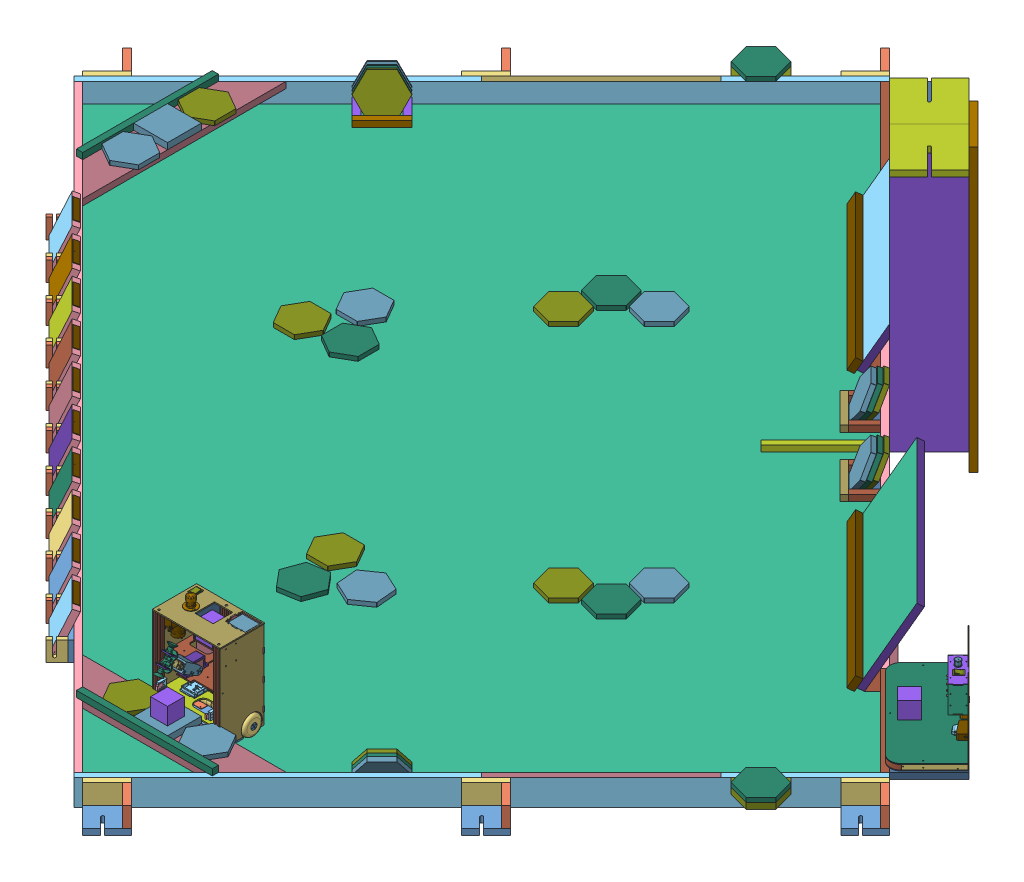
SolidWorks assembly conception_final_robot_autonome, configuration Default. Lengths in mm. (continued)
Components (placement in the parent): (continued)
- réplique-1: réplique [Default] at (173.8286 323.1947 656.2469) size (60 60 60)
- IBT-2 (module only)-1: IBT-2 (module only) [Default] at (112.5786 356.2835 564.3969) x (-1 0 0) z (0 0 1) size (51 40.62 49.7)
- IBT-2 (module only)-2: IBT-2 (module only) [Default] at (235.0786 361.6831 564.3969) size (51 40.62 49.7)
- support etage-1: support etage [Default] at (173.8286 272.8594 487.2468) x (1 0 0) z (0 1 0) size (19 14 15)
- support etage-2: support etage [Default] at (279.8286 272.9465 600.2469) x (-1 0 0) z (0 1 0) size (19 14 15)
- support etage-3: support etage [Default] at (67.8286 272.8594 600.2469) x (-1 0 0) z (0 1 0) size (19 14 15)
- réplique-3: réplique [Default] at (173.8286 480.6294 497.2468) size (60 60 60)
- support replique-1: support replique [Default] at (173.8286 446.6294 512.7469) x (-1 0 0) z (0 1 0) size (75 91 4)
- support etage-4: support etage [Default] at (173.8286 446.6294 487.2468) x (1 0 0) z (0 1 0) size (19 14 15)
- support etage-5: support etage [Default] at (163.8286 446.6294 477.2468) x (0 0 1) z (0 1 0) size (19 14 15)
- support etage-6: support etage [Default] at (183.8286 446.6294 477.2468) x (0 0 -1) z (0 1 0) size (19 14 15)
- support etage-7: support etage [Default] at (67.8286 379.2835 600.2469) x (-1 0 0) z (0 1 0) size (19 14 15)
- support etage-8: support etage [Default] at (279.8286 379.2835 600.2469) x (-1 0 0) z (0 1 0) size (19 14 15)
- support etage-9: support etage [Default] at (173.8286 379.2835 487.2468) x (1 0 0) z (0 1 0) size (19 14 15)
- etage lateral-1: etage lateral [Default] at (54.0286 394.8594 545.2469) x (0 0 -1) z (1 0 0) size (157 310 4)
- etage lateral-2: etage lateral [Default] at (289.6286 394.8594 545.2469) x (0 0 -1) z (1 0 0) size (157 310 4) (hidden)
- couvert arriere-1: couvert arriere [Default] at (184.7377 364.8594 463.2469) size (240 310 7)
- lipo battery-1: lipo battery [Default] at (255.0286 524.8594 497.2469) x (0 0 -1) z (0 -1 0) size (52 61 162)
- ventouse_final-1: ventouse_final [Default] at (157.7867 416.7859 702.1737) x (-0.271421 -0.541354 -0.79578) z (0.962461 -0.152666 -0.224416) size (30 42.25 32)
- ventouse_final-2: ventouse_final [Default] at (157.7867 490.4501 652.0613) x (-0.079274 0.560699 0.824216) z (0.996853 0.044589 0.065545) size (30 42.25 32)
- LM2596 DC to DC Buck Converter 3 A.STEP-1: LM2596 DC to DC Buck Converter 3 A.STEP [Default] at (274.0036 276.8594 498.8469) x (0 0 -1) z (1 0 0) size (43.2 15.15 21.25)
  - lm2596board.STEP-1: lm2596board.STEP [Default] at origin size (43.2 1.71 21.25)
  - smd100uF.STEP-1: smd100uF.STEP [Default] at (-17.25 2.55 0) x (0 0 -1) z (1 0 0) size (11.2 9.76 8.2)
  - smd220uF.STEP-1: smd220uF.STEP [Default] at (17.25 2.55 0) x (0 0 -1) z (1 0 0) size (11.2 9.76 8.2)
  - TrimmerW203.STEP-1: TrimmerW203.STEP [Default] at (4.6271 6.95 -9.1276) size (9.5 15.15 4.81)
  - smdS537diode.STEP-1: smdS537diode.STEP [Default] at (-9.35 1.75 8.875) x (-1 0 0) z (0 0 -1) size (6.5 2.06 2.5)
  - smdceramiccapacitor.STEP-1: smdceramiccapacitor.STEP [Default] at (-15 1.7 5.7969) x (0 0 1) z (-1 0 0) size (2.52 0.61 1.3)
  - smdceramiccapacitor.STEP-2: smdceramiccapacitor.STEP [Default] at (-1.3196 1.7 -5.2916) x (0 0 1) z (-1 0 0) size (2.52 0.61 1.3)
  - smdResistor331.STEP-1: smdResistor331.STEP [Default] at (-1.2696 1.7 -8.4665) x (0 0 1) z (-1 0 0) size (2.53 0.63 1.31)
  - smdResistor102.STEP-1: smdResistor102.STEP [Default] at (10.7771 1.7 -8.4665) x (0 0 -1) z (1 0 0) size (2.53 0.63 1.31)
  - smdLED.STEP-1: smdLED.STEP [Default] at (13.0521 1.75 -8.4701) x (0 0 -1) z (1 0 0) size (3.23 0.86 1.26)
  - smbInductor470.STEP-1: smbInductor470.STEP [Default] at (3.1271 2.1 3.175) size (12.5 7.41 12.5)
  - LM2596S.STEP-1: LM2596S.STEP [Default] at (-8.0627 1.8 -4.5407) size (9.8 4.61 14.95)
- e-stop 61-3440.stp-1: e-stop 61-3440.stp [Default] at (114.0286 514.8094 543.2469) x (-0.937891 0 -0.346929) z (0 1 0) size (43 43 76.4)
- couvert lateral replique-1: couvert lateral replique [Default] at (210.3286 485.7444 512.7469) x (0 0 1) z (-1 0 0) size (91 78.23 4)
- couvert lateral replique-2: couvert lateral replique [Default] at (141.3286 485.7444 512.7469) x (0 0 1) z (-1 0 0) size (91 78.23 4)
- profilé-1: profilé [Default] at (67.8286 364.8594 610.2469) x (1 0 0) z (0 -1 0) size (20 20 310)
- profilé-2: profilé [Default] at (279.8286 364.8594 610.2469) x (1 0 0) z (0 -1 0) size (20 20 310)
- profilé-3: profilé [Default] at (173.8286 364.8594 477.2469) x (1 0 0) z (0 -1 0) size (20 20 310)
- PompeVide-AirpoD2028B-12vdc-4: PompeVide-AirpoD2028B-12vdc [Défaut] at (77.3286 514.8594 552.1469) x (1 0 0) z (0 -1 0) size (38.6 62.4 92)
- roof-1: roof [Default] at (174.0286 528.8594 541.7469) x (1 0 0) z (0 -1 0) size (240 157 4)
- couvert lateral batterie-1: couvert lateral batterie [Default] at (216.0286 439.8594 497.2469) x (0 0 -1) z (1 0 0) size (63.8 174 4)
- couvert lateral batterie_2-1: couvert lateral batterie_2 [Default] at (255.0286 439.8594 531.2469) x (-1 0 0) z (0 0 -1) size (73.8 174 4)
- floor battery-1: floor battery [Default] at (252.5286 350.8594 497.0469) x (1 0 0) z (0 1 0) size (75.4 70.2 4)
- interrupteur principal-1: interrupteur principal [Défaut] at (76.5286 528.8594 489.2469) x (0 0 1) z (-1 0 0) size (32 33.35 25)
- support_ventouse-1: support_ventouse [Default] at (157.7867 440.3889 686.117) x (1 0 0) z (0 -0.826818 0.562469) size (35 26 4)
- support_ventouse-2: support_ventouse [Default] at (157.7867 470.1544 665.8681) x (1 0 0) z (0 -0.826818 0.562469) size (35 26 4)
- Assemblage1-1: Assemblage1 [Défaut] at (1585.9209 359.1947 -743.419) x (0.707107 0 0.707107) z (-0.707107 0 0.707107) size (440 246.17 210.2)
  - Pièce1-1: Pièce1 [Défaut] at origin size (440 156 3)
  - Pièce2-1: Pièce2 [Défaut] at (0 -85 105) x (-1 0 0) z (0 -1 0) size (439 210 3)
  - Part10 - Copie-1: Part10 - Copie [Default] at (-51.8676 -60.5031 49.9498) size (122.5 87.5 7.03)
  - Pièce9-1: Pièce9 [Défaut] at (-219.5 -76.5 104.5) x (0 0 -1) z (1 0 0) size (167 17 3)
  - Pièce6-2: Pièce6 [Défaut] at (-80 -76.5 207) size (359 17 3)
  - réplique-1: réplique [Default] at (0 -35 119.6611) size (60 60 60)
  - Pièce9-3: Pièce9 [Défaut] at (216.5 -76.5 104.5) x (0 0 -1) z (1 0 0) size (167 17 3)
  - Long Range SHARP IR Sensors - #GP2Y0A21YK0F-1: Long Range SHARP IR Sensors - #GP2Y0A21YK0F [Default] at (14.75 -35.3157 15.7) x (-1 0 0) z (0 0 1) size (44.5 18.9 13.5)
  - moraba3 3ordh-1: moraba3 3ordh [Défaut] at (-64.25 21.25 28) x (0 -1 0) z (1 0 0) size (93.5 53 3)
  - moraba3 3ordh-2: moraba3 3ordh [Défaut] at (61.25 21.25 27.8) x (0 -1 0) z (1 0 0) size (93.5 53 3)
  - moraba3 toul-2: moraba3 toul [Défaut] at (0 -25.5 28) x (1 0 0) z (0 1 0) size (128.5 53 3)
  - moraba3 toul loutaa-1: moraba3 toul loutaa [Défaut] at (0 65 28) x (1 0 0) z (0 1 0) size (128.5 53 3)
  - impr3d-1: impr3d [Défaut] at (0 -65 18) x (1 0 0) z (0 1 0) size (52 19 39.5)
  - FixAngle-1: FixAngle [Défaut] at (-216.5 -85 3) size (30 8 30)
  - FixAngle-2: FixAngle [Défaut] at (-61.25 -22.5 3) x (0 1 0) z (1 0 0) size (30 8 30)
  - FixAngle-3: FixAngle [Défaut] at (61.25 -22.5 3) x (-1 0 0) z (0 1 0) size (30 8 30)
  - FixAngle-4: FixAngle [Défaut] at (-61.25 65 3) x (1 0 0) z (0 -1 0) size (30 8 30)
  - FixAngle-5: FixAngle [Défaut] at (61.25 65 3) x (0 -1 0) z (-1 0 0) size (30 8 30)
  - FixAngle-9: FixAngle [Défaut] at (-61.25 -22.5 50.9) x (1 0 0) z (0 1 0) size (30 8 30)
  - FixAngle-10: FixAngle [Défaut] at (-61.25 65 50.9) x (0 -1 0) z (1 0 0) size (30 8 30)
  - FixAngle-11: FixAngle [Défaut] at (61.25 65 50.9) x (-1 0 0) z (0 -1 0) size (30 8 30)
  - FixAngle-12: FixAngle [Défaut] at (61.25 -22.5 50.9) x (0 1 0) z (-1 0 0) size (30 8 30)
  - arc_vitrine-1: arc_vitrine [Default] at (-219.5 -68 170) x (1 0 0) z (0 -1 0) size (50 50 17)
  - arc_vitrine-3: arc_vitrine [Default] at (179.5 -68 210) x (0 0 -1) z (0 -1 0) size (50 50 17)
  - support etage-1: support etage [Default] at (-216.5 -68 115) x (0 0 -1) z (0 1 0) size (19 14 15)
  - interrupteur principal-1: interrupteur principal [Défaut] at (13.25 68 26.5) x (0 0 -1) z (1 0 0) size (32 33.35 25)
  - FixAngle-13: FixAngle [Défaut] at (216.5 -85 3) x (0 0 1) z (-1 0 0) size (30 8 30)
  - support etage-3: support etage [Default] at (-77 -85 3) x (-1 0 0) z (0 -1 0) size (19 14 15)
  - support etage-4: support etage [Default] at (77 -85 3) x (-1 0 0) z (0 -1 0) size (19 14 15)
  - support etage-5: support etage [Default] at (216.5 -68 115) x (0 0 1) z (0 1 0) size (19 14 15)
  - Arduino UNO-1: Arduino UNO [Predeterminado] at (-140.4953 -85 41.7907) x (0 0 1) z (-1 0 0) size (74.8 15.1 53.3)
  - 5V One Channel Relay.step-1: 5V One Channel Relay.step [Default] at (-146.5 -85 84.8) x (0 0 1) z (-1 0 0) size (25.5 18.75 51)
  - support etage-6: support etage [Default] at (-22 -45.25 3) x (0 1 0) z (-1 0 0) size (19 14 15)
  - support etage-7: support etage [Default] at (22 -45.25 3) x (0 -1 0) z (1 0 0) size (19 14 15)
  - Force stop button-1: Force stop button [По умолчанию] at (-19.9998 66.9329 27.9999) x (0.906121 0 -0.423019) z (0 -1 0) size (20.79 20.79 48.92)
  - floor-1: floor [Default] at (0 -65 106.5) x (1 0 0) z (0 -1 0) size (439 207 3)
  - support etage-8: support etage [Default] at (0 -68 207) x (-1 0 0) z (0 1 0) size (19 14 15)
  - systeme de fixation-1: systeme de fixation [Défaut] at (0 -135 104.7444) x (-0.92707 0 -0.374889) z (-0.374889 0 0.92707) size (50.29 25 49.34)
  - fixation tige-1: fixation tige [Défaut] at (0 -85 104.7444) x (0.5 0 -0.866025) z (0.866025 0 0.5) size (13 55.5 15.01)
  - Long Range SHARP IR Sensors - #GP2Y0A21YK0F-2: Long Range SHARP IR Sensors - #GP2Y0A21YK0F [Default] at (122.0333 -35.3157 24.7506) x (-0.992278 0 -0.124035) z (-0.124035 0 0.992278) size (44.5 18.9 13.5)
  - support sharp lateral-1: support sharp lateral [Default] at (107.2359 -41.8157 3) size (60 20 29.34)
  - support sharp lateral-2: support sharp lateral [Default] at (-107.2359 -41.8157 3) x (-1 0 0) z (0 0 1) size (60 20 29.34)
  - Long Range SHARP IR Sensors - #GP2Y0A21YK0F-3: Long Range SHARP IR Sensors - #GP2Y0A21YK0F [Default] at (-92.7611 -35.3157 21.0916) x (-0.992278 0 0.124035) z (0.124035 0 0.992278) size (44.5 18.9 13.5)
- system wheel-1: system wheel [Default] at (267.4597 228.3737 520.7342) x (0 -0.852789 -0.522255) z (1 0 0) size (69.5 69.5 30.5)
  - part1-1: part1 [Default] at (0.5601 15.4113 33.6689) size (21.5 21.5 11)
  - part2-1: part2 [Default] at (0.5601 15.4113 5.1689) x (0 1 0) z (0 0 -1) size (21.5 21.5 18)
  - _gomme-1: _gomme [Default] at (0.5601 15.4113 11.6689) size (69.5 69.5 22)
- switch-1: switch [Default] at (84.2286 310.6027 623.2469) x (0 1 0) z (1 0 0) size (14 24 6)
- support_switch-1: support_switch [Default] at (77.8286 298.3527 609.7469) x (0 0 1) z (0 -1 0) size (29 9 24.5)
- switch-2: switch [Default] at (263.4286 310.6027 623.2469) x (0 -1 0) z (-1 0 0) size (14 24 6)
- support_switch-2: support_switch [Default] at (269.8286 322.8527 609.7469) x (0 0 1) z (0 1 0) size (29 9 24.5)
- system wheel-2: system wheel [Default] at (80.1976 227.4184 520.1492) x (0 0.852789 0.522255) z (-1 0 0) size (69.5 69.5 30.5)
  - part1-1: part1 [Default] at (0.5601 15.4113 33.6689) size (21.5 21.5 11)
  - part2-1: part2 [Default] at (0.5601 15.4113 5.1689) x (0 1 0) z (0 0 -1) size (21.5 21.5 18)
  - _gomme-1: _gomme [Default] at (0.5601 15.4113 11.6689) size (69.5 69.5 22)
- BillePorteuse-1: BillePorteuse [Défaut] at (173.8286 208.7594 609.7469) x (-0.837169 0 -0.546944) z (-0.546944 0 0.837169) size (31 21 31)
- etage lateral-3: etage lateral [Default] at (289.6286 394.8594 545.2469) x (0 0 -1) z (1 0 0) size (157 310 4)
- Baterijas testeris.step-1: Baterijas testeris.step [Default] at (200.7286 409.8594 471.7469) x (0 -1 0) z (1 0 0) size (41 12 24.1)
Mates (geometry in assembly coordinates):
- Coincident33: coincident anti-aligned: plane of étage 3-1 through (169.8286 383.2835 544.2469) normal (0 1 0); plane of Servo-1 through (150.2867 383.2835 566.2469) normal (0 -1 0)
- Concentric1: concentric anti-aligned: cylinder of Servo-1 through (146.7867 399.2835 597.2469) axis (1 0 0) radius 9.5; cylinder of bras_replique-1 through (146.7867 399.2835 597.2469) axis (-1 0 0) radius 12.5
- Coincident66: coincident anti-aligned: plane of Servo-1 through (146.7867 399.2835 597.2469) normal (-1 0 0); plane of bras_replique-1 through (146.7867 399.2835 597.2469) normal (1 0 0)
- Width3: width anti-aligned: plane of ##Servo_MG_996R-3 through (147.7867 431.8506 662.8986) normal (-1 0 0); plane of bras_replique-1 through (187.7867 431.8506 662.8986) normal (1 0 0); plane of ##Servo_MG_996R-3 through (146.7867 399.2835 597.2469) normal (1 0 0); plane of bras_replique-1 through (188.7867 399.2835 597.2469) normal (-1 0 0)
- Width4: width anti-aligned: plane of ##Servo_MG_996R-3 through (187.7867 431.8506 662.8986) normal (0 -0.826818 0.562469); plane of bras_replique-1 through (187.7867 448.3869 651.6492) normal (0 0.826818 -0.562469); plane of ##Servo_MG_996R-3 through (146.7867 412.5126 588.2474) normal (0 0.826818 -0.562469); plane of bras_replique-1 through (146.7867 386.0544 606.2464) normal (0 -0.826818 0.562469)
- Coincident67: coincident anti-aligned: plane of ##Servo_MG_996R-3 through (167.7867 435.844 650.9901) normal (0 -0.562469 -0.826818); plane of bras_replique-1 through (146.7867 435.844 650.9901) normal (0 0.562469 0.826818)
- Concentric5: concentric aligned: cylinder of ##Servo_MG_996R-3 through (157.7867 444.3373 663.475) axis (0 -0.562469 -0.826818) radius 3; cylinder of Access_HS-645_BrasRondPetitModele-1 through (157.7867 442.6499 660.9946) axis (0 -0.562469 -0.826818) radius 2.75
- Coincident71: coincident anti-aligned: plane of ##Servo_MG_996R-3 through (157.7867 444.3373 663.475) normal (0 0.562469 0.826818); plane of Access_HS-645_BrasRondPetitModele-1 through (160.5367 444.3373 663.475) normal (0 -0.562469 -0.826818)
- Width5: width anti-aligned: plane of support servo kbyr-1 through (151.5367 383.2835 566.2469) normal (0 0 1); plane of support servo kbyr-1 through (151.5367 405.2835 609.2469) normal (0 0 -1); plane of Servo-1 through (150.2867 383.2835 566.2469) normal (0 0 -1); plane of Servo-1 through (150.2867 383.2835 609.2469) normal (0 0 1)
- Width6: width aligned: plane of support servo kbyr-1 through (181.5367 409.2835 603.2469) normal (1 0 0); plane of support servo kbyr-1 through (151.5367 409.2835 603.2469) normal (-1 0 0); plane of Servo-1 through (182.7867 399.2835 587.7469) normal (1 0 0); plane of Servo-1 through (150.2867 399.2835 587.7469) normal (-1 0 0)
- Coincident75: coincident anti-aligned: plane of Servo-1 through (150.2867 415.2835 566.2469) normal (0 1 0); plane of support servo kbyr-1 through (151.5367 415.2835 566.2469) normal (0 -1 0)
- Distance1: distance = 15 mm: plane of support servo kbyr-1 through (151.5367 409.2835 614.2469) normal (0 0 1); plane of étage 3-1 through (289.8286 383.2835 629.2469) normal (0 0 1)
- Distance2: distance = 3 mm anti-aligned: plane of robot_sghyr-1/base_robot_sghyr-1 through (173.8286 209.8594 547.2469) normal (0 -1 0); plane of TABLE_2021.step-1/BaseTable.step-1/Ground.step-1 through (-179.7247 201.1947 -780.8956) normal (0 1 0)
- Distance3: distance = 3 mm anti-aligned: plane of étage 3-1 through (289.8286 383.2835 629.2469) normal (0 0 1); plane of TABLE_2021.step-1/Distributeurs.step-1/DistributeurCoin_1.step-1/Taquet.step-1 through (534.4531 249.1947 626.2469) normal (0 0 -1)
- Width7: width anti-aligned: plane of étage 3-1 through (289.8286 383.2835 467.2469) normal (1 0 0); plane of étage 3-1 through (57.8286 383.2835 467.2469) normal (-1 0 0); plane of TABLE_2021.step-1/Distributeurs.step-1/DistributeurCoin_1.step-1/SupportStatuette.step-1 through (113.8286 271.1947 626.2469) normal (-1 0 0); plane of TABLE_2021.step-1/Distributeurs.step-1/DistributeurCoin_1.step-1/SupportStatuette.step-1 through (233.8286 271.1947 746.2469) normal (1 0 0)
- Coincident81: coincident anti-aligned: plane of TABLE_2021.step-1/Distributeurs.step-1/DistributeurCoin_1.step-1/SupportStatuette.step-1 through (173.8286 293.1947 686.2469) normal (0 1 0); plane of réplique-1 through (143.8286 293.1947 716.2469) normal (0 -1 0)
- Width8: width anti-aligned: plane of réplique-1 through (203.8286 353.1947 716.2469) normal (1 0 0); plane of réplique-1 through (143.8286 353.1947 716.2469) normal (-1 0 0); plane of TABLE_2021.step-1/Distributeurs.step-1/DistributeurCoin_1.step-1/SupportStatuette.step-1 through (113.8286 271.1947 626.2469) normal (-1 0 0); plane of TABLE_2021.step-1/Distributeurs.step-1/DistributeurCoin_1.step-1/SupportStatuette.step-1 through (233.8286 271.1947 746.2469) normal (1 0 0)
- Width9: width aligned: plane of réplique-1 through (173.8286 323.1947 656.2469) normal (0 0 -1); plane of réplique-1 through (173.8286 323.1947 716.2469) normal (0 0 1); plane of TABLE_2021.step-1/Distributeurs.step-1/DistributeurCoin_1.step-1/Taquet.step-1 through (534.4531 249.1947 626.2469) normal (0 0 -1); plane of TABLE_2021.step-1/Distributeurs.step-1/DistributeurCoin_1.step-1/Taquet (1).step-1 through (414.4531 271.1947 746.2469) normal (0 0 -1)
- Parallel1: parallel aligned: plane of étage 3-1 through (169.8286 379.2835 544.2469) normal (0 -1 0); plane of IBT-2 (module only)-1 through (112.5786 354.6835 564.3969) normal (0 -1 0)
- Coincident87: coincident anti-aligned: plane of étage 3-1 through (169.8286 379.2835 544.2469) normal (0 -1 0); plane of IBT-2 (module only)-1 through (107.5231 379.2835 582.5719) normal (0 1 0)
- Parallel2: parallel aligned: plane of étage 3-1 through (57.8286 383.2835 467.2469) normal (-1 0 0); plane of IBT-2 (module only)-1 through (87.0786 356.2835 582.5719) normal (-1 0 0)
- Distance6: distance = 30 mm aligned: plane of étage 3-1 through (57.8286 383.2835 467.2469) normal (-1 0 0); plane of IBT-2 (module only)-1 through (87.8286 354.6835 586.7569) normal (-1 0 0)
- Width12: width aligned: plane of support etage-1 through (171.4786 257.8594 485.7468) normal (-1 0 0); plane of robot_sghyr-1/profilé-1 through (176.1786 257.8594 485.7468) normal (1 0 0); plane of support etage-1 through (168.3286 514.8594 483.8075) normal (0.707107 0 0.707107); plane of robot_sghyr-1/profilé-1 through (179.3286 514.8594 483.8075) normal (-0.707107 0 0.707107)
- Coincident90: coincident anti-aligned: plane of robot_sghyr-1/profilé-1 through (183.4286 514.8594 487.2468) normal (0 0 1); plane of support etage-1 through (183.3286 257.8594 487.2468) normal (0 0 -1)
- Coincident91: coincident anti-aligned: plane of robot_sghyr-1/etage electronique-1 through (173.8286 272.8594 547.2469) normal (0 -1 0); plane of support etage-1 through (183.3286 272.8594 487.2468) normal (0 1 0)
- Coincident94: coincident anti-aligned: plane of robot_sghyr-1/etage electronique-1 through (173.8286 272.8594 547.2469) normal (0 -1 0); plane of support etage-3 through (58.3286 272.8594 600.2469) normal (0 1 0)
- Width15: width aligned: plane of support replique-1 through (184.3286 450.6294 467.2469) normal (-1 0 0); plane of support replique-1 through (163.3286 450.6294 488.2469) normal (1 0 0); plane of robot_sghyr-1/profilé-1 through (163.8286 514.8594 486.8468) normal (-1 0 0); plane of robot_sghyr-1/profilé-1 through (183.8286 514.8594 486.8468) normal (1 0 0)
- Parallel3: parallel anti-aligned: plane of robot_sghyr-1/profilé-1 through (179.9286 514.8594 475.743) normal (0 1 0); plane of support replique-1 through (173.8286 466.6326 512.7469) normal (0 -1 0)
- Coincident95: coincident: plane of robot_sghyr-1/profilé-1 through (183.4286 514.8594 467.2468) normal (0 0 -1); plane of support replique-1 through (206.3286 470.6326 467.2469) normal (0 0 -1)
- Width18: width aligned: plane of support etage-6 through (182.3286 451.6326 479.5968) normal (0 0 1); plane of support etage-6 through (182.3286 451.6326 474.8968) normal (0 0 -1); plane of robot_sghyr-1/profilé-1 through (183.4286 514.8594 467.2468) normal (0 0 -1); plane of robot_sghyr-1/profilé-1 through (183.4286 514.8594 487.2468) normal (0 0 1)
- Coincident100: coincident anti-aligned: plane of robot_sghyr-1/profilé-1 through (183.8286 514.8594 486.8468) normal (1 0 0); plane of support etage-6 through (183.8286 451.6326 467.7468) normal (-1 0 0)
- Width19: width anti-aligned: plane of réplique-3 through (203.8286 510.6294 557.2468) normal (1 0 0); plane of réplique-3 through (143.8286 510.6294 557.2468) normal (-1 0 0); plane of support replique-1 through (141.3286 450.6294 558.2469) normal (-1 0 0); plane of support replique-1 through (206.3286 450.6294 558.2469) normal (1 0 0)
- Coincident102: coincident anti-aligned: plane of réplique-3 through (143.8286 450.6294 557.2468) normal (0 -1 0); plane of support replique-1 through (173.8286 450.6294 512.7469) normal (0 1 0)
- Coincident104: coincident anti-aligned: plane of étage 3-1 through (169.8286 379.2835 544.2469) normal (0 -1 0); plane of support etage-7 through (58.3286 379.2835 600.2469) normal (0 1 0)
- Coincident106: coincident anti-aligned: plane of étage 3-1 through (169.8286 379.2835 544.2469) normal (0 -1 0); plane of support etage-8 through (270.3286 379.2835 600.2469) normal (0 1 0)
- Width22: width anti-aligned: plane of support etage-9 through (176.1786 364.2835 485.7468) normal (1 0 0); plane of support etage-9 through (171.4786 364.2835 485.7468) normal (-1 0 0); plane of robot_sghyr-1/profilé-1 through (183.8286 514.8594 486.8468) normal (1 0 0); plane of robot_sghyr-1/profilé-1 through (163.8286 514.8594 486.8468) normal (-1 0 0)
- Coincident107: coincident anti-aligned: plane of robot_sghyr-1/profilé-1 through (164.2286 514.8594 487.2468) normal (0 0 1); plane of support etage-9 through (183.3286 364.2835 487.2468) normal (0 0 -1)
- Coincident108: coincident anti-aligned: plane of étage 3-1 through (169.8286 379.2835 544.2469) normal (0 -1 0); plane of support etage-9 through (183.3286 379.2835 487.2468) normal (0 1 0)
- Width23: width anti-aligned: plane of étage 3-1 through (57.8286 383.2835 467.2469) normal (-1 0 0); plane of étage 3-1 through (289.8286 383.2835 467.2469) normal (1 0 0); plane of robot_sghyr-1/base_robot_sghyr-1 through (258.8286 209.8594 537.2469) normal (1 0 0); plane of robot_sghyr-1/base_robot_sghyr-1 through (88.8286 209.8594 537.2469) normal (-1 0 0)
- Coincident112: coincident anti-aligned: plane of robot_sghyr-1/base_robot_sghyr-1 through (173.8286 214.8594 547.2469) normal (0 1 0); plane of etage lateral-1 through (58.0286 214.8594 620.2469) normal (0 -1 0)
- Coincident114: coincident aligned: plane of robot_sghyr-1/profilé-1 through (183.4286 514.8594 467.2468) normal (0 0 -1); plane of étage 3-1 through (289.8286 384.2835 467.2469) normal (0 0 -1)
- Coincident115: coincident anti-aligned: plane of robot_sghyr-1/base_robot_sghyr-1 through (173.8286 214.8594 547.2469) normal (0 1 0); plane of couvert arriere-1 through (53.8286 214.8594 467.2469) normal (0 -1 0)
- Coincident116: coincident aligned: plane of robot_sghyr-1/base_robot_sghyr-1 through (53.8286 214.8594 462.2469) normal (-1 0 0); plane of couvert arriere-1 through (53.8286 544.8594 467.2469) normal (-1 0 0)
- Coincident117: coincident anti-aligned: plane of couvert arriere-1 through (184.7377 364.8594 467.2469) normal (0 0 1); plane of robot_sghyr-1/profilé-1 through (183.4286 514.8594 467.2468) normal (0 0 -1)
- Coincident120: coincident anti-aligned: plane of robot_sghyr-1/etage electronique-1 through (173.8286 276.8594 547.2469) normal (0 1 0); plane of LM2596 DC to DC Buck Converter 3 A.STEP-1/lm2596board.STEP-1 through (274.0036 276.8594 498.8469) normal (0 -1 0)
- Distance7: distance = 5 mm anti-aligned: plane of LM2596 DC to DC Buck Converter 3 A.STEP-1/lm2596board.STEP-1 through (284.6286 278.5594 520.4469) normal (1 0 0); plane of etage lateral-2 through (289.6286 394.8594 545.2469) normal (-1 0 0)
- Distance8: distance = 10 mm anti-aligned: plane of couvert arriere-1 through (184.7377 364.8594 467.2469) normal (0 0 1); plane of LM2596 DC to DC Buck Converter 3 A.STEP-1/lm2596board.STEP-1 through (284.6286 278.5594 477.2469) normal (0 0 -1)
- Distance9: distance = 10 mm anti-aligned: plane of robot_sghyr-1/profilé-1 through (183.4286 514.8594 487.2468) normal (0 0 1); plane of réplique-3 through (173.8286 500.6326 497.2468) normal (0 0 -1)
- Coincident127: coincident anti-aligned: plane of couvert arriere-1 through (184.7377 364.8594 467.2469) normal (0 0 1); plane of couvert lateral replique-1 through (206.3286 524.8594 467.2469) normal (0 0 -1)
- Coincident130: coincident anti-aligned: plane of support replique-1 through (206.3286 450.6294 558.2469) normal (1 0 0); plane of couvert lateral replique-1 through (206.3286 485.7444 512.7469) normal (-1 0 0)
- Concentric9: concentric anti-aligned: cylinder of robot_sghyr-1/base_robot_sghyr-1 through (67.8286 214.8594 610.2469) axis (0 -1 0) radius 2.5; cylinder of profilé-1 through (67.8286 214.8594 610.2469) axis (0 1 0) radius 2.5
- Coincident131: coincident anti-aligned: plane of robot_sghyr-1/base_robot_sghyr-1 through (173.8286 214.8594 547.2469) normal (0 1 0); plane of profilé-1 through (66.3248 214.8594 616.3469) normal (0 -1 0)
- Concentric10: concentric anti-aligned: cylinder of robot_sghyr-1/base_robot_sghyr-1 through (173.8286 214.8594 477.2469) axis (0 -1 0) radius 2.5; cylinder of profilé-3 through (173.8286 214.8594 477.2469) axis (0 1 0) radius 2.5
- Coincident132: coincident anti-aligned: plane of robot_sghyr-1/base_robot_sghyr-1 through (173.8286 214.8594 547.2469) normal (0 1 0); plane of profilé-3 through (172.3248 214.8594 483.3469) normal (0 -1 0)
- Coincident133: coincident aligned: plane of etage lateral-2 through (293.6286 544.8594 620.2469) normal (0 0 1); plane of profilé-2 through (289.4286 214.8594 620.2469) normal (0 0 1)
- Coincident137: coincident anti-aligned: plane of etage lateral-2 through (289.6286 394.8594 545.2469) normal (-1 0 0); plane of couvert arriere-1 through (289.6286 255.0594 467.2469) normal (1 0 0)
- Coincident138: coincident aligned: plane of etage lateral-2 through (293.6286 544.8594 463.2469) normal (0 0 -1); plane of couvert arriere-1 through (184.7377 364.8594 463.2469) normal (0 0 -1)
- Coincident139: coincident anti-aligned: plane of robot_sghyr-1/etage electronique-1 through (289.8286 272.8594 467.2469) normal (0 0 -1); plane of couvert arriere-1 through (184.7377 364.8594 467.2469) normal (0 0 1)
- Coincident148: coincident anti-aligned: plane of PompeVide-AirpoD2028B-12vdc-1 through (289.6286 475.8594 595.2469) normal (1 0 0); plane of etage lateral-2 through (289.6286 394.8594 545.2469) normal (-1 0 0)
- Distance12: distance = 5 mm anti-aligned: plane of PompeVide-AirpoD2028B-12vdc-1 through (251.0286 475.8594 595.2469) normal (0 0 1); plane of profilé-2 through (270.2286 214.8594 600.2469) normal (0 0 -1)
- Coincident154: coincident anti-aligned: plane of profilé-1 through (66.3248 524.8594 616.3469) normal (0 1 0); plane of roof-1 through (174.0286 524.8594 541.7469) normal (0 -1 0)
- Coincident155: coincident aligned: plane of etage lateral-1 through (54.0286 394.8594 545.2469) normal (-1 0 0); plane of roof-1 through (54.0286 524.8594 620.2469) normal (-1 0 0)
- Coincident156: coincident aligned: plane of profilé-1 through (77.4286 214.8594 620.2469) normal (0 0 1); plane of roof-1 through (54.0286 524.8594 620.2469) normal (0 0 1)
- Width27: width anti-aligned: plane of roof-1 through (216.0286 524.8594 487.2469) normal (0 0 1); plane of roof-1 through (220.0286 524.8594 507.2469) normal (0 0 -1); plane of couvert lateral batterie-1 through (220.0286 528.8594 487.3469) normal (0 0 -1); plane of couvert lateral batterie-1 through (220.0286 524.8594 507.1469) normal (0 0 1)
- Coincident157: coincident anti-aligned: plane of roof-1 through (216.0286 524.8594 507.2469) normal (1 0 0); plane of couvert lateral batterie-1 through (216.0286 439.8594 497.2469) normal (-1 0 0)
- Coincident158: coincident aligned: plane of roof-1 through (174.0286 528.8594 541.7469) normal (0 1 0); plane of couvert lateral batterie-1 through (220.0286 528.8594 507.1469) normal (0 1 0)
- Width28: width anti-aligned: plane of couvert lateral batterie_2-1 through (264.9286 524.8594 527.2469) normal (1 0 0); plane of couvert lateral batterie_2-1 through (245.1286 528.8594 527.2469) normal (-1 0 0); plane of roof-1 through (245.0286 524.8594 531.2469) normal (1 0 0); plane of roof-1 through (265.0286 524.8594 527.2469) normal (-1 0 0)
- Coincident159: coincident aligned: plane of roof-1 through (174.0286 528.8594 541.7469) normal (0 1 0); plane of couvert lateral batterie_2-1 through (264.9286 528.8594 527.2469) normal (0 1 0)
- Coincident160: coincident anti-aligned: plane of roof-1 through (265.0286 524.8594 531.2469) normal (0 0 -1); plane of couvert lateral batterie_2-1 through (255.0286 439.8594 531.2469) normal (0 0 1)
- Width29: width aligned: plane of lipo battery-1 through (224.5286 362.8594 523.2469) normal (-1 0 0); plane of lipo battery-1 through (285.5286 362.8594 523.2469) normal (1 0 0); plane of roof-1 through (290.0286 524.8594 467.2469) normal (-1 0 0); plane of roof-1 through (220.0286 524.8594 507.2469) normal (1 0 0)
- Width30: width aligned: plane of roof-1 through (220.0286 524.8594 467.2469) normal (0 0 1); plane of roof-1 through (220.0286 524.8594 527.2469) normal (0 0 -1); plane of lipo battery-1 through (285.5286 362.8594 523.2469) normal (0 0 1); plane of lipo battery-1 through (285.5286 362.8594 471.2469) normal (0 0 -1)
- Concentric11: concentric aligned: cylinder of e-stop 61-3440.stp-1 through (114.0286 532.9094 543.2469) axis (0 1 0) radius 12; cylinder of roof-1 through (114.0286 524.8594 543.2469) axis (0 1 0) radius 7.5
- Coincident161: coincident anti-aligned: plane of e-stop 61-3440.stp-1 through (114.0286 528.8594 543.2469) normal (0 -1 0); plane of roof-1 through (174.0286 528.8594 541.7469) normal (0 1 0)
- Distance13: distance = 4 mm aligned: plane of lipo battery-1 through (255.0286 524.8594 497.2469) normal (0 1 0); plane of roof-1 through (174.0286 528.8594 541.7469) normal (0 1 0)
- Distance14: distance = 40 mm aligned: plane of IBT-2 (module only)-2 through (212.8286 363.2831 589.2469) normal (0 0 1); plane of étage 3-1 through (289.8286 383.2835 629.2469) normal (0 0 1)
- Coincident163: coincident anti-aligned: plane of couvert lateral batterie_2-1 through (289.9286 354.8594 527.2469) normal (0 -1 0); plane of floor battery-1 through (252.5286 354.8594 497.0469) normal (0 1 0)
- Coincident164: coincident aligned: plane of couvert lateral batterie-1 through (216.0286 439.8594 497.2469) normal (-1 0 0); plane of floor battery-1 through (216.0286 354.8594 467.2469) normal (-1 0 0)
- Coincident165: coincident anti-aligned: plane of couvert arriere-1 through (184.7377 364.8594 467.2469) normal (0 0 1); plane of floor battery-1 through (216.0286 354.8594 467.2469) normal (0 0 -1)
- Coincident166: coincident anti-aligned: plane of roof-1 through (174.0286 528.8594 541.7469) normal (0 1 0); plane of interrupteur principal-1 through (76.5286 528.8594 489.2469) normal (0 -1 0)
- Parallel4: parallel anti-aligned: plane of roof-1 through (54.0286 524.8594 620.2469) normal (-1 0 0); plane of interrupteur principal-1 through (89.0286 530.8594 473.2469) normal (1 0 0)
- Distance15: distance = 10 mm aligned: plane of interrupteur principal-1 through (64.0286 530.8594 473.2469) normal (0 0 -1); plane of roof-1 through (54.0286 524.8594 463.2469) normal (0 0 -1)
- Distance16: distance = 10 mm aligned: plane of interrupteur principal-1 through (64.0286 530.8594 473.2469) normal (-1 0 0); plane of roof-1 through (54.0286 524.8594 620.2469) normal (-1 0 0)
- Coincident173: coincident anti-aligned: plane of support_ventouse-1 through (162.7867 430.8945 679.2719) normal (0 -0.562469 -0.826818); plane of SUPPORT VENTOUSE-1 through (147.1896 426.7604 682.0842) normal (0 0.562469 0.826818)
- Concentric12: concentric anti-aligned: cylinder of ventouse_final-1 through (157.7867 416.7859 702.1737) axis (0 -0.826818 0.562469) radius 6.5; cylinder of support_ventouse-1 through (157.7867 437.0816 688.3669) axis (0 0.826818 -0.562469) radius 6.5
- Coincident174: coincident anti-aligned: plane of ventouse_final-1 through (157.7867 437.0816 688.3669) normal (0 0.826818 -0.562469); plane of support_ventouse-1 through (157.7867 437.0816 688.3669) normal (0 -0.826818 0.562469)
- Coincident175: coincident anti-aligned: plane of SUPPORT VENTOUSE-1 through (157.7867 442.9311 661.408) normal (-1 0 0); plane of support_ventouse-1 through (157.7867 440.3889 686.117) normal (1 0 0)
- Width31: width anti-aligned: plane of SUPPORT VENTOUSE-1 through (144.776 418.1266 678.282) normal (0 -0.826818 0.562469); plane of SUPPORT VENTOUSE-1 through (144.776 467.7357 644.5339) normal (0 0.826818 -0.562469); plane of bras_replique-1 through (146.7867 412.5126 588.2474) normal (0 0.826818 -0.562469); plane of bras_replique-1 through (146.7867 386.0544 606.2464) normal (0 -0.826818 0.562469)
- Concentric13: concentric aligned: cylinder of ventouse_final-2 through (157.7867 490.4501 652.0613) axis (0 0.826818 -0.562469) radius 6.5; cylinder of support_ventouse-2 through (157.7867 466.8471 668.118) axis (0 0.826818 -0.562469) radius 6.5
- Distance18: distance = 10 mm aligned: plane of support_ventouse-1 through (157.7867 437.0816 688.3669) normal (0 -0.826818 0.562469); plane of SUPPORT VENTOUSE-1 through (144.776 418.1266 678.282) normal (0 -0.826818 0.562469)
- Coincident181: coincident anti-aligned: plane of ventouse_final-2 through (157.7867 470.1544 665.8681) normal (0 -0.826818 0.562469); plane of support_ventouse-2 through (157.7867 470.1544 665.8681) normal (0 0.826818 -0.562469)
- Coincident182: coincident anti-aligned: plane of TABLE_2021.step-1/BaseTable.step-1/ExperimentZone.step-2 through (1515.2102 271.1947 -672.7083) normal (0 1 0); plane of Assemblage1-1/Pièce2-1 through (1511.6747 271.1947 -669.1728) normal (0 -1 0)
- Coincident184: coincident aligned: plane of TABLE_2021.step-1/BaseTable.step-1/ExperimentZone.step-2 through (1589.4564 271.1947 -739.8834) normal (0.707107 0 -0.707107); plane of Assemblage1-1/Pièce1-1 through (1585.9209 359.1947 -743.419) normal (0.707107 0 -0.707107)
- Width35: width anti-aligned: plane of TABLE_2021.step-1/BaseTable.step-1/ExperimentZone.step-2 through (1745.0199 271.1947 -584.32) normal (0.707107 0 0.707107); plane of Assemblage1-1/Pièce9-1 through (1285.4005 271.1947 -761.0966) normal (-0.707107 0 -0.707107); plane of TABLE_2021.step-1/BaseTable.step-1/ExperimentZone.step-2 through (1356.8183 282.6947 -824.7363) normal (-0.707107 0 -0.707107); plane of Assemblage1-1/Pièce9-2 through (1667.2382 350.1947 -513.6093) normal (0.707107 0 0.707107)
- Concentric14: concentric aligned: cylinder of ##Servo_MG_996R-3 through (157.7867 444.3373 663.475) axis (0 -0.562469 -0.826818) radius 3; cylinder of Access_HS-645_BrasRondPetitModele-1 through (157.7867 442.6499 660.9946) axis (0 -0.562469 -0.826818) radius 4.5
- Coincident187: coincident anti-aligned: plane of SUPPORT VENTOUSE-1 through (157.7867 442.9311 661.408) normal (-1 0 0); plane of Access_HS-645_BrasRondPetitModele-1 through (157.7867 442.6499 660.9946) normal (1 0 0)
- Coincident188: coincident anti-aligned: plane of SUPPORT VENTOUSE-1 through (135.3298 469.9855 647.8412) normal (0 -0.562469 -0.826818); plane of Access_HS-645_BrasRondPetitModele-1 through (161.5367 445.181 664.7152) normal (0 0.562469 0.826818)
- Concentric15: concentric aligned: cylinder of robot_sghyr-1/pololu-37D-encoder-1 through (273.8286 235.8594 507.2469) axis (-1 0 0) radius 3; cylinder of system wheel-1/accoupelement court-1 through (272.8286 235.8594 507.2469) axis (-1 0 0) radius 3
- Coincident189: coincident anti-aligned: plane of profilé-1 through (77.8286 214.8594 619.8469) normal (1 0 0); plane of support_switch-1 through (77.8286 322.8527 619.2469) normal (-1 0 0)
- Width39: width aligned: plane of switch-1 through (85.8286 317.6027 632.2469) normal (0 1 0); plane of switch-1 through (85.8286 303.6027 632.2469) normal (0 -1 0); plane of support_switch-1 through (77.8286 322.8527 619.2469) normal (0 1 0); plane of support_switch-1 through (77.8286 298.3527 619.2469) normal (0 -1 0)
- Parallel5: parallel aligned: plane of switch-1 through (85.8286 303.6027 614.2469) normal (0 0 -1); plane of support_switch-1 through (77.8286 298.3527 600.2469) normal (0 0 -1)
- Distance20: distance = 6 mm aligned: plane of robot_sghyr-1/base_robot_sghyr-1 through (293.8286 214.8594 632.2469) normal (0 0 1); plane of switch-1 through (89.8286 303.6027 638.2469) normal (0 0 1)
- Coincident191: coincident anti-aligned: plane of switch-1 through (83.8286 310.6027 623.2469) normal (-1 0 0); plane of support_switch-1 through (83.8286 322.8527 619.2469) normal (1 0 0)
- Coincident192: coincident aligned: plane of profilé-1 through (77.4286 214.8594 600.2469) normal (0 0 -1); plane of support_switch-1 through (77.8286 298.3527 600.2469) normal (0 0 -1)
- Distance21: distance = 2 mm anti-aligned: plane of system wheel-1/accoupelement court-2 through (260.8286 235.9447 507.2991) normal (-1 0 0); plane of robot_sghyr-1/pololu-37D-encoder-1 through (258.8286 235.8594 507.2469) normal (1 0 0)
- Tangent1: tangent: plane of TABLE_2021.step-1/BaseTable.step-1/Ground.step-1 through (-179.7247 201.1947 -780.8956) normal (0 1 0); circle of system wheel-2/_gomme-1
- Concentric16: concentric aligned: cylinder of étage 3-1 through (174.5367 379.2835 621.2469) axis (0 1 0) radius 2.5; cylinder of support servo kbyr-1 through (174.5367 383.2835 621.2469) axis (0 1 0) radius 2
- Parallel6: parallel anti-aligned: plane of robot_sghyr-1/base_robot_sghyr-1 through (173.8286 209.8594 547.2469) normal (0 -1 0); plane of TABLE_2021.step-1/BaseTable.step-1/Ground.step-1 through (-179.7247 201.1947 -780.8956) normal (0 1 0)
- Concentric17: concentric aligned: cylinder of robot_sghyr-1/Robot2015_support bille porteuse-1 through (173.8286 226.8594 609.7469) axis (0 -1 0) radius 11.9; cylinder of BillePorteuse-1 through (173.8286 201.2594 609.7469) axis (0 -1 0) radius 12
- Coincident193: coincident anti-aligned: plane of robot_sghyr-1/Robot2015_support bille porteuse-1 through (173.8286 210.7594 609.7469) normal (0 -1 0); plane of BillePorteuse-1 through (183.8747 210.7594 616.3102) normal (0 1 0)
- Coincident198: coincident: plane of couvert lateral replique-1 through (206.3286 524.8594 467.2469) normal (0 1 0); plane of roof-1 through (174.0286 524.8594 541.7469) normal (0 -1 0)
- Coincident200: coincident anti-aligned: plane of couvert lateral replique-1 through (206.3286 524.8594 467.2469) normal (0 1 0); plane of roof-1 through (174.0286 524.8594 541.7469) normal (0 -1 0)
- Coincident201: coincident aligned: plane of support replique-1 through (173.8286 446.6294 512.7469) normal (0 -1 0); plane of couvert lateral replique-1 through (206.3286 446.6294 467.2469) normal (0 -1 0)
- Coincident202: coincident aligned: plane of support replique-1 through (206.3286 450.6294 558.2469) normal (0 0 1); plane of couvert lateral replique-1 through (206.3286 524.8594 558.2469) normal (0 0 1)
- Coincident203: coincident anti-aligned: plane of support replique-1 through (173.8286 446.6294 512.7469) normal (0 -1 0); plane of support etage-4 through (183.3286 446.6294 487.2468) normal (0 1 0)
- Concentric18: concentric anti-aligned: cylinder of support replique-1 through (173.8286 450.6294 496.2468) axis (0 -1 0) radius 1.6; cylinder of support etage-4 through (173.8286 431.6294 496.2468) axis (0 1 0) radius 1.6
- Coincident204: coincident anti-aligned: plane of support replique-1 through (173.8286 446.6294 512.7469) normal (0 -1 0); plane of support etage-6 through (183.8286 446.6294 467.7468) normal (0 1 0)
- Concentric19: concentric anti-aligned: cylinder of support replique-1 through (192.8286 450.6294 477.2468) axis (0 -1 0) radius 1.6; cylinder of support etage-6 through (192.8286 431.6294 477.2468) axis (0 1 0) radius 1.6
- Coincident207: coincident anti-aligned: plane of support replique-1 through (173.8286 446.6294 512.7469) normal (0 -1 0); plane of support etage-5 through (163.8286 446.6294 486.7468) normal (0 1 0)
- Concentric20: concentric anti-aligned: cylinder of support replique-1 through (154.8286 450.6294 477.2468) axis (0 -1 0) radius 1.6; cylinder of support etage-5 through (154.8286 431.6294 477.2468) axis (0 1 0) radius 1.6
- Coincident208: coincident anti-aligned: plane of couvert arriere-1 through (184.7377 364.8594 467.2469) normal (0 0 1); plane of Baterijas testeris.step-1 through (200.7286 409.8594 467.2469) normal (0 0 -1)
- Width40: width anti-aligned: plane of Baterijas testeris.step-1 through (212.7286 424.8594 467.2469) normal (1 0 0); plane of couvert arriere-1 through (188.7286 424.8594 467.2469) normal (-1 0 0); plane of Baterijas testeris.step-1 through (213.2286 424.8594 460.2469) normal (-1 0 0); plane of couvert arriere-1 through (188.2286 424.8594 460.2469) normal (1 0 0)
- Coincident209: coincident anti-aligned: plane of couvert arriere-1 through (188.2286 424.8594 460.2469) normal (0 -1 0); plane of Baterijas testeris.step-1 through (212.7286 424.8594 467.2469) normal (0 1 0)
- Concentric21: concentric anti-aligned: cylinder of étage 3-1 through (158.5367 379.2835 621.2469) axis (0 1 0) radius 2.5; cylinder of support servo kbyr-1 through (158.5367 396.2835 621.2469) axis (0 -1 0) radius 3
